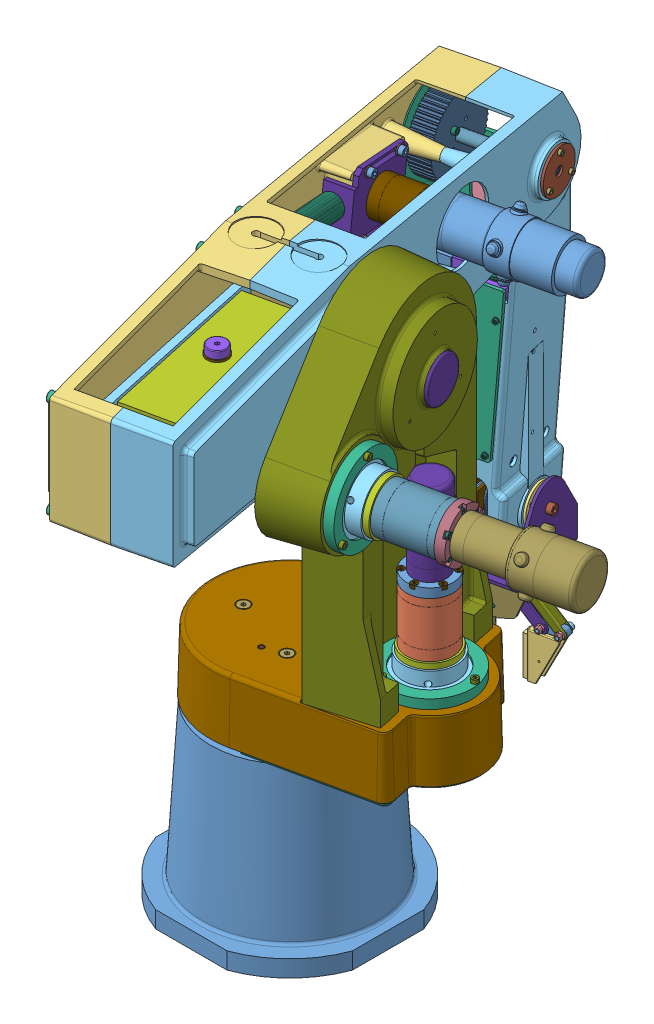
SolidWorks assembly Robot, configuration Défaut. Lengths in mm. (continued)
Components (placement in the parent): (continued)
- SE-AvtBras-1: SE-AvtBras [Défaut] at (-61.3918 532.5 -273.1877) x (0 1 0) z (-0.977211 0 0.212271) size (419.1 115.2 105.3)
  - AvtBrasD-1: AvtBrasD [Défaut] at origin size (406.26 90.38 52)
  - AvtBrasG-1: AvtBrasG [Défaut] at (-0.1665 0.8325 0) size (406.15 90.36 52)
  - parallel pin hardened_iso-1: parallel pin hardened_iso [Goupille  - 4 x 16 - A - St] at (-265.5 30.1675 -8) x (0 0 1) z (-0.010471 -0.999945 0) size (16 4 4)
  - Vis C HC, M 6x70-1: Vis C HC, M 6x70 [Défaut] at (-65 -16 45.5) x (1 0 0) z (0 -1 0) size (10 76 10)
  - GoupillePosition-1: GoupillePosition [Défaut] at (-65 -16 0.2) x (0 0 1) z (-0.991523 0.129934 0) size (10 8 8)
  - Support moteur-1: Support moteur [Défaut] at (-98.931 38.4675 -40.5) x (0 0 1) z (1 0 0) size (77 78 106)
  - socket head cap screw_iso-1: socket head cap screw_iso [Vis CHC M5 x 12 --- 12N] at (-173.5 -4.3325 -27.8) x (0 0 -1) z (0.120643 0.992696 0) size (17 8.5 8.5)
  - socket head cap screw_iso-2: socket head cap screw_iso [Vis CHC M5 x 12 --- 12N] at (-153.5 -4.3325 -27.8) x (0 0 -1) z (0.975756 0.218862 0) size (17 8.5 8.5)
  - plain washer large grade ac_iso-1: plain washer large grade ac_iso [Rondelle M5 Washer ISO 7093 - 5] at (-173.5 -4.3325 -32.8) x (0 0 1) z (-1 0 0) size (1.2 15 15)
  - plain washer large grade ac_iso-3: plain washer large grade ac_iso [Rondelle M5 Washer ISO 7093 - 5] at (-153.5 -4.3325 -32.8) x (0 0 1) z (-1 0 0) size (1.2 15 15)
  - Poulie_M300-006-1: Poulie_M300-006 [Défaut] at (0 0 39) x (0 0 1) z (-0.707107 -0.707107 0) size (22 81.46 81.46)
  - Goupille Cylindrique type A  , 4x24-1: Goupille Cylindrique type A  , 4x24 [Défaut] at (9.1924 9.1924 26.3203) x (0.697271 -0.716808 0) z (0 0 1) size (4 4 24)
  - Goupille Cylindrique type A  , 4x24-3: Goupille Cylindrique type A  , 4x24 [Défaut] at (-9.1924 -9.1924 24.7225) x (-0.993131 -0.117006 0) z (0 0 1) size (4 4 24)
  - socket head cap screw_iso-3: socket head cap screw_iso [Vis CHC M4 x 25 ] at (-9.1924 9.1924 20) x (0 0 1) z (-1 0 0) size (29 7 7)
  - socket head cap screw_iso-4: socket head cap screw_iso [Vis CHC M4 x 25 ] at (9.1924 -9.1924 20) x (0 0 1) z (-1 0 0) size (29 7 7)
  - Came M300 008-1: Came M300 008 [Default] at (0 0 -43) x (0.999885 0.015178 0) z (0 0 1) size (76.42 80 10)
  - parallel pin hardened_iso-2: parallel pin hardened_iso [Goupille  - 4 x 16 - A - St] at (-6.5 -11.2583 -51.3276) x (0 0 1) z (-0.969957 0.243275 0) size (16 4 4)
  - socket head cap screw_iso-5: socket head cap screw_iso [CHC M4 x 16 --- 16N] at (-12.9985 -0.1973 -29) x (0 0 -1) z (-0.999639 0.026878 0) size (20 7 7)
  - socket head cap screw_iso-10: socket head cap screw_iso [CHC M4 x 16 --- 16N] at (6.6701 -11.1584 -29) x (0 0 -1) z (-0.999639 0.026878 0) size (20 7 7)
  - socket head cap screw_iso-12: socket head cap screw_iso [CHC M4 x 16 --- 16N] at (6.3284 11.3557 -29) x (0 0 -1) z (-0.999639 0.026878 0) size (20 7 7)
  - plain washer small grade a_iso-1: plain washer small grade a_iso [Washer M 4] at (-265.5 -21.8325 -8) x (0 0 1) z (-1 0 0) size (0.5 8 8)
  - socket head cap screw_iso-18: socket head cap screw_iso [CHC M4 x 16 --- 16N] at (-265.5 -21.8325 -12.5) x (0 0 1) z (-1 0 0) size (20 7 7)
  - plain washer small grade a_iso-3: plain washer small grade a_iso [Washer M 4] at (-265.5 23.1675 -8) x (0 0 1) z (-1 0 0) size (0.5 8 8)
  - socket head cap screw_iso-19: socket head cap screw_iso [CHC M4 x 16 --- 16N] at (-265.5 23.1675 -12.5) x (0 0 1) z (-1 0 0) size (20 7 7)
  - plain washer small grade a_iso-5: plain washer small grade a_iso [Washer M 4] at (-43.253 27.1675 -8) x (0 0 1) z (-1 0 0) size (0.5 8 8)
  - socket head cap screw_iso-20: socket head cap screw_iso [CHC M4 x 16 --- 16N] at (-43.253 27.1675 -12.5) x (0 0 1) z (-1 0 0) size (20 7 7)
  - moteur poignet-1: moteur poignet [Défaut] at (-218.4709 19.4675 19.5) size (70.8 35 35)
  - socket head cap screw_iso-21: socket head cap screw_iso [ISO 4762 M2 x 6 --- 6N] at (-174.931 8.4675 19.5) x (-1 0 0) z (0 0.924225 0.381849) size (8 3.8 3.8)
  - socket head cap screw_iso-22: socket head cap screw_iso [ISO 4762 M2 x 6 --- 6N] at (-174.931 19.4675 8.5) x (-1 0 0) z (0 -0.381849 0.924225) size (8 3.8 3.8)
  - socket head cap screw_iso-23: socket head cap screw_iso [ISO 4762 M2 x 6 --- 6N] at (-174.931 30.4675 19.5) x (-1 0 0) z (0 -0.924225 -0.381849) size (8 3.8 3.8)
  - socket head cap screw_iso-24: socket head cap screw_iso [ISO 4762 M2 x 6 --- 6N] at (-174.931 19.4675 30.5) x (-1 0 0) z (0 0.381849 -0.924225) size (8 3.8 3.8)
  - Vis CS, M 4x55-1: Vis CS, M 4x55 [Défaut] at (-88.5 -0.5325 -38.5) x (0 -1 0) z (0 0 1) size (7 57.41 7)
  - hex thin nut gradeb_iso-1: hex thin nut gradeb_iso [Hexagon Nut ISO - 4036 - M4 - N] at (-96.731 -0.5325 -38.5) x (0 -0.306361 -0.951915) z (1 0 0) size (7 8.08 2.2)
  - Accouplement flexible-1: Accouplement flexible [Default] at (-161.451 19.4675 19.5) x (-1 0 0) z (0 0.117803 -0.993037) size (17.76 9.53 9.53)
  - Codeur poignet-1: Codeur poignet [Défaut] at (-230.631 -7.9406 32.9669) x (0 0.056728 -0.99839) z (1 0 0) size (30 41.1 18.3)
  - Réducteur-1: Réducteur [Défaut] at (-143.931 29.4675 5.5) x (1 0 0) z (0 0 -1) size (82 70 28)
  - radial ball bearing_68_iso-1: radial ball bearing_68_iso [RBB - 1810 - 14,SI,NC,14_68] at (-317.5 -0.8325 -38.5) x (0 0 1) z (-0.812829 -0.582503 0) size (5 19 19)
  - plain washer small grade a_iso-6: plain washer small grade a_iso [Washer courte m5 7092 - 5] at (-138.931 7.4675 33.5) x (0 0 -1) z (1 0 0) size (1 9 9)
  - socket head cap screw_iso-25: socket head cap screw_iso [vis chc M5 x 35 --- 22N] at (-138.931 7.4675 39.5) x (0 0 -1) z (0.75446 0.656346 0) size (40 8.5 8.5)
  - plain washer small grade a_iso-7: plain washer small grade a_iso [Washer courte m5 7092 - 5] at (-88.931 7.4675 33.5) x (0 0 -1) z (1 0 0) size (1 9 9)
  - plain washer small grade a_iso-8: plain washer small grade a_iso [Washer courte m5 7092 - 5] at (-88.931 -35.5325 33.5) x (0 0 -1) z (1 0 0) size (1 9 9)
  - socket head cap screw_iso-26: socket head cap screw_iso [vis chc M5 x 35 --- 22N] at (-88.931 7.4675 39.5) x (0 0 -1) z (0.75446 0.656346 0) size (40 8.5 8.5)
  - socket head cap screw_iso-27: socket head cap screw_iso [vis chc M5 x 35 --- 22N] at (-88.931 -35.5325 39.5) x (0 0 -1) z (0.75446 0.656346 0) size (40 8.5 8.5)
  - Couvercle-3: Couvercle [Défaut] at (-317.5 -0.8325 -49.8) x (-0.559761 -0.828654 0) z (-0.828654 0.559761 0) size (41 8.8 41)
  - socket head cap screw_iso-28: socket head cap screw_iso [Vis CHC M3x8] at (-310.5 11.2918 -52.8) x (0 0 1) z (-0.923728 -0.383049 0) size (11 5.5 5.5)
  - socket head cap screw_iso-29: socket head cap screw_iso [Vis CHC M3x8] at (-310.5 -12.9569 -52.8) x (0 0 1) z (0.130134 0.991496 0) size (11 5.5 5.5)
  - socket head cap screw_iso-30: socket head cap screw_iso [Vis CHC M3x8] at (-331.5 -0.8325 -52.8) x (0 0 1) z (0.793594 -0.608447 0) size (11 5.5 5.5)
  - radial ball bearing_68_iso-4: radial ball bearing_68_iso [RBB - 1810 - 14,SI,NC,14_68] at (-317.5 -0.8325 38.2) x (0 0 1) z (-0.978908 -0.204302 0) size (5 19 19)
  - Couvercle-4: Couvercle [Défaut] at (-317.5 -0.8325 49.5) x (0.997516 0.070441 0) z (-0.070441 0.997516 0) size (41 8.8 41)
  - socket head cap screw_iso-31: socket head cap screw_iso [Vis CHC M3x8] at (-310.5 11.2918 52.5) x (0 0 -1) z (1 0 0) size (11 5.5 5.5)
  - socket head cap screw_iso-32: socket head cap screw_iso [Vis CHC M3x8] at (-331.5 -0.8325 52.5) x (0 0 -1) z (-0.5 0.866025 0) size (11 5.5 5.5)
  - socket head cap screw_iso-33: socket head cap screw_iso [Vis CHC M3x8] at (-310.5 -12.9569 52.5) x (0 0 -1) z (-0.5 -0.866025 0) size (11 5.5 5.5)
  - Capot Superieur_plexi-1: Capot Superieur_plexi [Défaut] at (-81.8928 43.8087 0) x (1 0 0) z (0 1 0) size (220 89.9 3.57)
  - plain washer 10673 type snl_iso-1: plain washer 10673 type snl_iso [rondelle M2] at (-264 46.4087 28) x (0 -1 0) z (0 0 1) size (0.6 6 6)
  - socket head cap screw_iso-34: socket head cap screw_iso [ISO 4762 M2.5 x 10 --- 10N] at (-264 48.9087 28) x (0 -1 0) z (0 0 1) size (12.5 4.5 4.5)
  - plain washer 10673 type snl_iso-9: plain washer 10673 type snl_iso [rondelle M2] at (-264 46.4087 -28) x (0 -1 0) z (0 0 1) size (0.6 6 6)
  - plain washer 10673 type snl_iso-11: plain washer 10673 type snl_iso [rondelle M2] at (-54 46.4087 -40) x (0 -1 0) z (0 0 1) size (0.6 6 6)
  - plain washer 10673 type snl_iso-13: plain washer 10673 type snl_iso [rondelle M2] at (-54 46.4087 40) x (0 -1 0) z (0 0 1) size (0.6 6 6)
  - socket head cap screw_iso-35: socket head cap screw_iso [ISO 4762 M2.5 x 10 --- 10N] at (-264 48.9087 -28) x (0 -1 0) z (0 0 1) size (12.5 4.5 4.5)
  - socket head cap screw_iso-36: socket head cap screw_iso [ISO 4762 M2.5 x 10 --- 10N] at (-54 48.9087 -40) x (0 -1 0) z (0 0 1) size (12.5 4.5 4.5)
  - socket head cap screw_iso-37: socket head cap screw_iso [ISO 4762 M2.5 x 10 --- 10N] at (-54 48.9087 40) x (0 -1 0) z (0 0 1) size (12.5 4.5 4.5)
  - Capot inferieur_plexi-1: Capot inferieur_plexi [Défaut] at (-207.8847 -47.4738 0) x (1 0 0) z (0 1 0) size (165 92.79 3.62)
  - plain washer 10673 type snl_iso-14: plain washer 10673 type snl_iso [rondelle M2] at (-121.3236 -48.0738 -40) x (0 1 0) z (-1 0 0) size (0.6 6 6)
  - plain washer 10673 type snl_iso-16: plain washer 10673 type snl_iso [rondelle M2] at (-121.3236 -48.0738 40) x (0 1 0) z (-1 0 0) size (0.6 6 6)
  - plain washer 10673 type snl_iso-18: plain washer 10673 type snl_iso [rondelle M2] at (-251.3236 -48.0738 30) x (0 1 0) z (-1 0 0) size (0.6 6 6)
  - plain washer 10673 type snl_iso-20: plain washer 10673 type snl_iso [rondelle M2] at (-251.3236 -48.0738 -30) x (0 1 0) z (-1 0 0) size (0.6 6 6)
  - socket head cap screw_iso-38: socket head cap screw_iso [ISO 4762 M2.5 x 10 --- 10N] at (-251.3236 -50.5738 -30) x (0 1 0) z (0 0 1) size (12.5 4.5 4.5)
  - socket head cap screw_iso-39: socket head cap screw_iso [ISO 4762 M2.5 x 10 --- 10N] at (-251.3236 -50.5738 30) x (0 1 0) z (0 0 -1) size (12.5 4.5 4.5)
  - socket head cap screw_iso-40: socket head cap screw_iso [ISO 4762 M2.5 x 10 --- 10N] at (-121.3236 -50.5738 40) x (0 1 0) z (0 0 -1) size (12.5 4.5 4.5)
  - socket head cap screw_iso-41: socket head cap screw_iso [ISO 4762 M2.5 x 10 --- 10N] at (-121.3236 -50.5738 -40) x (0 1 0) z (0 0 -1) size (12.5 4.5 4.5)
  - radial ball bearing_68_skf-1: radial ball bearing_68_skf [Roulement à billes 618-8] at (-113.931 -10.5325 -32.5) x (0 0 -1) z (1 0 0) size (4 16 16)
  - Arbre réducteur-1: Arbre réducteur [Défaut] at (-113.931 -10.5325 33.5) size (8 8 68)
  - Entretoise-1: Entretoise [Défaut] at (-113.931 -10.5325 -10.5) size (12 12 16)
- Arbre moteur Lacet-1: Arbre moteur Lacet [Défaut] at (122.0871 255.5 -29.1721) x (0 -1 0) z (-0.495579 0 0.868563) size (78.5 36.84 36.92)
  - entraineur-1: entraineur [Défaut] at origin size (78.5 20 20)
  - PoulieE lacet-1: PoulieE lacet [Défaut] at (49 0 0) x (0 -1 0) z (-1 0 0) size (36.84 36.92 30)
  - socket set screw flat point_iso-1: socket set screw flat point_iso [ISO 4026 - M8 x 10-N] at (49 0 16.5) x (0 0 -1) z (1 0 0) size (10 8 8)
  - socket set screw flat point_iso-2: socket set screw flat point_iso [ISO 4026 - M8 x 10-N] at (-7.2554 0 12.9535) x (0 0 -1) z (0.96252 -0.271209 0) size (10 8 8)
- A-M_Epaule-1: A-M_Epaule [Défaut] at (143.3488 474.5 66.3524) x (-0.977211 0 0.212271) z (-0.212271 0 -0.977211) size (78.5 36.84 36.92)
  - entraineur-1: entraineur [Défaut] at origin size (78.5 20 20)
  - P-E_Epaule-1: P-E_Epaule [Défaut] at (49 0 0) x (0 -1 0) z (-1 0 0) size (36.84 36.92 30)
  - socket set screw flat point_iso-1: socket set screw flat point_iso [ISO 4026 - M8 x 10-N] at (49 0 16.5) x (0 0 -1) z (1 0 0) size (10 8 8)
  - socket set screw flat point_iso-2: socket set screw flat point_iso [ISO 4026 - M8 x 10-N] at (-7.2554 0 12.9535) x (0 0 -1) z (0.96252 -0.271209 0) size (10 8 8)
- Poulie_M300-007-1: Poulie_M300-007 [Défaut] at (-55.3873 549.2909 -151.3264) x (0.977211 0 -0.212271) z (0.17106 -0.592111 0.787492) size (27 22.5 22.65)
- Poulie Poignet-1: Poulie Poignet [Défaut] at (-39.1232 418.569 -267.2467) x (-0.212271 0 -0.977211) z (0.977211 0 -0.212271) size (27.43 27.43 20)
- poulie pivotement poignet-1: poulie pivotement poignet [Défaut] at (-76.1895 174.3879 -240.3141) x (-0.99945 0 0.033175) z (0 -1 0) size (20 20 14)
- Support_poignet-1: Support_poignet [Défaut] at (-61.215 215 -272.3741) x (0 1 0) z (-0.977211 0 0.212271) size (98.66 84.05 127)
  - Support-1: Support [Défaut] at origin size (81.5 81.2 115)
  - Assemblage axe pince-1: Assemblage axe pince [Défaut] at (-13.5 0 0) x (0 0 -1) z (1 0 0) size (109 40 59)
    - partie centrale axe avant bras-1: partie centrale axe avant bras [Défaut] at origin size (12 40 21)
    - intérieur pièce centrale-1: intérieur pièce centrale [Défaut] at (-3 1.5 5) size (6 15.94 13)
    - intérieur pièce centrale-2: intérieur pièce centrale [Défaut] at (3 -1.5 5) x (-1 0 0) z (0 0 1) size (6 15.94 13)
    - coté axe avant bras-1: coté axe avant bras [Défaut] at (-6 1.807 8.3053) x (1 0 0) z (0 0.944488 0.328546) size (48.5 11 11)
    - coté axe avant bras-2: coté axe avant bras [Défaut] at (6 -1.6292 8.2468) x (-1 0 0) z (0 -0.95512 0.296219) size (48.5 11 11)
    - axe roulements-1: axe roulements [Défaut] x (0 0 -1) z (0.989499 0.144542 0) size (38 10.89 10.89)
  - Assemblage support moteur-1: Assemblage support moteur [Défaut] at (-44.3507 -38.7833 30.5386) x (-1 0 0) z (0 0 -1) size (78.32 60.15 22.52)
    - Support moteur + axe-1: Support moteur + axe [Défaut] at origin size (75.82 60.15 22.2)
    - capteur sur support moteur-1: capteur sur support moteur [Défaut] at (-40.0112 47.5459 15.95) x (0 -0.781659 -0.623706) z (1 0 0) size (6.5 6.5 27.6)
    - plaque avant support moteur-1: plaque avant support moteur [Défaut] at (14.8869 1.1807 -1.9) x (0 0 -1) z (1 0 0) size (22 24 2.5)
  - Ecrou hexagonal ISO 4032, M 9-1: Ecrou hexagonal ISO 4032, M 9 [Défaut] at (-44.23 0 0) x (0 1 0) z (0 0 1) size (16.17 6.98 14)
  - moteur pivotement poignet-1: moteur pivotement poignet [Défaut] at (-26.4843 -28.1507 21.4386) x (-1 0 0) z (0 -0.157023 -0.987595) size (81.2 19.59 19.59)
    - réducteur micromoteur-1: réducteur micromoteur [Défaut] at origin size (48.3 16 16)
    - micromoteur-1: micromoteur [Défaut] at (-2.1408 0 0) x (1 0 0) z (0 -0.965969 0.258658) size (41 16 16)
  - Poulie axe poignet-1: Poulie axe poignet [Défaut] at (0 0 -18.0612) x (-0.954858 -0.297063 0) z (0 0 -1) size (58.99 58.99 20)
  - Vis C HC, M 6x16-1: Vis C HC, M 6x16 [Défaut] at (0 0 57.5) x (0.243653 -0.969862 0) z (-0.969862 -0.243653 0) size (10 22.04 10)
  - Vis C HC, M 6x16-2: Vis C HC, M 6x16 [Défaut] at (0 0 -57.5) x (1 0 0) z (0 1 0) size (10 22.04 10)
- PortePince-1: PortePince [Défaut] at (-61.215 215 -272.3741) x (0 1 0) z (0.212271 0 0.977211) size (147.79 157.25 45.47)
  - Corps_poignet-1: Corps_poignet [Défaut] at (-113.4 0 -8.5) x (0 -1 0) z (0 0 1) size (87.98 118.07 45.47)
    - Main-1: Main [Défaut] at origin size (87.98 81.17 33)
    - fourreau de poignet-1: fourreau de poignet [Défaut] at (0 76.4 8.5) x (0 1 0) z (0.435216 0 0.900326) size (46.9 34.05 34.05)
    - Roulement type BC 9x17x4-1: Roulement type BC 9x17x4 [Défaut] at (0 94.9 8.5) x (0 -1 0) z (-0.453716 0 0.891146) size (4 17 17)
    - Roulement type BC 9x17x4-2: Roulement type BC 9x17x4 [Défaut] at (0 71.1711 8.5) x (0 -1 0) z (0 0 1) size (4 17 17)
    - Axe-goupille-1: Axe-goupille [Défaut] at (36.5 37 17) size (3.5 3.5 17)
    - Axe-goupille-2: Axe-goupille [Défaut] at (18.5 37 17) size (3.5 3.5 17)
    - Axe-goupille-3: Axe-goupille [Défaut] at (-18.5 37 17) size (3.5 3.5 17)
    - Axe-goupille-4: Axe-goupille [Défaut] at (-36.5 37 17) size (3.5 3.5 17)
    - Axe-goupille-5: Axe-goupille [Défaut] at (-12.5 10 17) size (3.5 3.5 17)
    - Axe-goupille-6: Axe-goupille [Défaut] at (12.5 10 17) size (3.5 3.5 17)
  - bielle 1-1: bielle 1 [Défaut] at (-106.9547 -75.1317 5.4) x (-0.717304 0.69676 0) z (0 0 -1) size (9.87 58.75 10.8)
  - bielle 1-2: bielle 1 [Défaut] at (-106.9547 75.1317 -5.4) x (-0.717304 -0.69676 0) z (0 0 1) size (9.87 58.75 10.8)
  - bielle 2-1: bielle 2 [Défaut] at (-80.8832 -14.1453 5.4) x (0.717304 -0.69676 0) z (0 0 -1) size (12.5 61.5 10.8)
    - bielle 2-1: bielle 2 [Défaut] at origin size (12.5 61.5 10.8)
    - goupille bielle 2-1: goupille bielle 2 [Défaut] at (6.25 18 10.8) x (-0.698934 -0.715186 0) z (0 0 1) size (3.5 3.5 10.8)
  - bielle 2-2: bielle 2 [Défaut] at (-80.8832 14.1453 -5.4) x (0.717304 0.69676 0) z (0 0 1) size (12.5 61.5 10.8)
    - bielle 2-1: bielle 2 [Défaut] at origin size (12.5 61.5 10.8)
    - goupille bielle 2-1: goupille bielle 2 [Défaut] at (6.25 18 10.8) x (-0.698934 -0.715186 0) z (0 0 1) size (3.5 3.5 10.8)
  - Mors-3: Mors [Défaut] at (-210.2541 103.6501 -0.5) x (-1 0 0) z (0 0 -1) size (60 39.8 20)
    - Bielle 3-1: Bielle 3 [Défaut] at (-104.4629 -50.0022 -4.6) size (9.5 27.5 8.2)
    - goupille-1: goupille [Défaut] at (-106.9629 -37.5022 -0.5) x (0 -0.527582 0.849504) z (-1 0 0) size (4 4 14)
    - mors-1: mors [Défaut] at (-49.5801 -64.5882 6.5) size (48 34 14)
    - ecrou_uni_7474-m4x0_7-4_8-5s-1: ecrou_uni_7474-m4x0_7-4_8-5s [Défaut] at (-99.7129 -32.0022 4.9) x (0.66757 0.744547 0) z (0 0 1) size (7 8.09 4.8)
    - ecrou_uni_7474-m4x0_7-4_8-5s-2: ecrou_uni_7474-m4x0_7-4_8-5s [Défaut] at (-99.7129 -50.0022 4.9) x (0.967807 0.251692 0) z (0 0 1) size (7 8.09 4.8)
    - vis chc M4x16-1: vis chc M4x16 [Default] at (-99.7129 -32.0022 -5.9) x (0.255972 0.966684 0) z (0 0 1) size (7 7 20)
    - vis chc M4x16-2: vis chc M4x16 [Default] at (-99.7129 -50.0022 -5.9) x (-0.658187 0.752854 0) z (0 0 1) size (7 7 20)
    - Vis Chc M4-1: Vis Chc M4 [Default] at (-92.9629 -44.5022 -0.5) x (0 0 1) z (-1 0 0) size (7 7 16)
  - Mors-4: Mors [Défaut] at (-210.2541 -103.6501 0.5) x (-1 0 0) z (0 0 1) size (60 39.8 20)
    - Bielle 3-1: Bielle 3 [Défaut] at (-104.4629 -50.0022 -4.6) size (9.5 27.5 8.2)
    - goupille-1: goupille [Défaut] at (-106.9629 -37.5022 -0.5) x (0 -0.527582 0.849504) z (-1 0 0) size (4 4 14)
    - mors-1: mors [Défaut] at (-49.5801 -64.5882 6.5) size (48 34 14)
    - ecrou_uni_7474-m4x0_7-4_8-5s-1: ecrou_uni_7474-m4x0_7-4_8-5s [Défaut] at (-99.7129 -32.0022 4.9) x (0.66757 0.744547 0) z (0 0 1) size (7 8.09 4.8)
    - ecrou_uni_7474-m4x0_7-4_8-5s-2: ecrou_uni_7474-m4x0_7-4_8-5s [Défaut] at (-99.7129 -50.0022 4.9) x (0.967807 0.251692 0) z (0 0 1) size (7 8.09 4.8)
    - vis chc M4x16-1: vis chc M4x16 [Default] at (-99.7129 -32.0022 -5.9) x (0.255972 0.966684 0) z (0 0 1) size (7 7 20)
    - vis chc M4x16-2: vis chc M4x16 [Default] at (-99.7129 -50.0022 -5.9) x (-0.658187 0.752854 0) z (0 0 1) size (7 7 20)
    - Vis Chc M4-1: Vis Chc M4 [Default] at (-92.9629 -44.5022 -0.5) x (0 0 1) z (-1 0 0) size (7 7 16)
Mates (geometry in assembly coordinates):
- Coaxiale1: concentric aligned: cylinder of Ens_Socle-1/Fourreau_200-604-1 through (0 221.7474 0) axis (0 1 0) radius 23.5; cylinder of SE_Chaise-1/SE-Assise-1/SKF_7204-2 through (0 165.3625 0) axis (0 1 0) radius 23.5
- Coïncidente1: coincident anti-aligned: plane of Ens_Socle-1/Fourreau_200-604-1 through (-1.9708 229.5 23.4172) normal (0 -1 0); plane of SE_Chaise-1/SE-Assise-1/SKF_7204-1 through (20.3016 229.5 -4.4099) normal (0 1 0)
- Coaxiale2: concentric anti-aligned: cylinder of SE_Chaise-1/Dossier-1 through (63.5173 532.5 -13.7908) axis (0.977211 0 -0.212271) radius 23.5; cylinder of Bras-1/AXE_Bras-1/7204_Rlt-Billes-2 through (137.9197 532.5 -29.9526) axis (-0.977211 0 0.212271) radius 23.5
- Coïncidente2: coincident anti-aligned: plane of SE_Chaise-1/Dossier-1 through (124.593 532.5 -27.0578) normal (-0.977211 0 0.212271); plane of Bras-1/AXE_Bras-1/7204_Rlt-Billes-2 through (127.5156 548.0575 -13.6033) normal (0.977211 0 -0.212271)
- Coaxiale3: concentric aligned: cylinder of Bras-1/AXE 04 021 M300 011-1 through (-121.9788 532.5 -260.0268) axis (0.977211 0 -0.212271) radius 6; cylinder of SE-AvtBras-1/AvtBrasG-1 through (-112.2067 532.5 -262.1496) axis (0.977211 0 -0.212271) radius 6
- Coïncidente3: coincident aligned: plane of Bras-1/BrasDroit-2 through (-0.5391 505.7717 6.953) normal (-0.977211 0 0.212271); plane of SE-AvtBras-1/AvtBrasD-1 through (-61.3918 532.5 -273.1877) normal (-0.977211 0 0.212271)
- Coaxiale5: concentric aligned: cylinder of SE_Chaise-1/Moto-réducteur lacet-1/SKF 6002-1 through (122.0871 209.2625 -29.1721) axis (0 1 0) radius 7.5; cylinder of Arbre moteur Lacet-1/entraineur-1 through (122.0871 277.7027 -29.1721) axis (0 1 0) radius 7.5
- Coïncidente5: coincident anti-aligned: plane of SE_Chaise-1/Moto-réducteur lacet-1/SKF 6002-2 through (127.3321 255.5 -23.3989) normal (0 1 0); plane of Arbre moteur Lacet-1/entraineur-1 through (130.7727 255.5 -24.2163) normal (0 -1 0)
- Coaxiale6: concentric aligned: cylinder of SE_Chaise-1/Moteur Epaule-1/SKF 6002-2 through (98.165 474.5 76.1673) axis (0.977211 0 -0.212271) radius 7.5; cylinder of A-M_Epaule-1/entraineur-1 through (165.0455 474.5 61.6395) axis (0.977211 0 -0.212271) radius 7.5
- Coïncidente6: coincident anti-aligned: plane of SE_Chaise-1/Moteur Epaule-1/SKF 6002-1 through (144.9823 473.2287 73.8728) normal (0.977211 0 -0.212271); plane of A-M_Epaule-1/entraineur-1 through (143.3488 484.5 66.3524) normal (-0.977211 0 0.212271)
- Coaxiale7: concentric anti-aligned: cylinder of Bras-1/MotoReduc_Coude-1/Sortie reduc-1 through (-54.8986 549.2909 -151.4325) axis (0.977211 0 -0.212271) radius 5; cylinder of Poulie_M300-007-1 through (-67.3627 549.2909 -148.725) axis (-0.977211 0 0.212271) radius 5
- Coaxiale8: concentric aligned: cylinder of Bras-1/MotoReduc_Coude-1/Sortie reduc-1 through (-71.8779 552.2514 -151.8675) axis (0.17106 -0.592111 0.787492) radius 1.5; cylinder of Poulie_M300-007-1 through (-72.9599 555.9965 -156.8484) axis (0.17106 -0.592111 0.787492) radius 1.5
- Coaxiale9: concentric aligned: cylinder of SE-AvtBras-1/Arbre réducteur-1 through (-25.4422 418.569 -270.2185) axis (-0.977211 0 0.212271) radius 4; cylinder of Poulie Poignet-1 through (-29.3511 418.569 -269.3694) axis (-0.977211 0 0.212271) radius 4
- Coïncidente7: coincident anti-aligned: plane of SE-AvtBras-1/Entretoise-1 through (-48.8953 418.569 -265.124) normal (0.977211 0 -0.212271); plane of Poulie Poignet-1 through (-48.8953 418.569 -265.124) normal (-0.977211 0 0.212271)
- Coaxiale10: concentric anti-aligned: cylinder of Support_poignet-1/Assemblage axe pince-1/axe roulements-1 through (-61.215 163.5 -272.3741) axis (0 1 0) radius 4.5; cylinder of PortePince-1/Corps_poignet-1/fourreau de poignet-1 through (-61.215 146.4624 -272.3741) axis (0 -1 0) radius 11
- Coaxiale11: concentric anti-aligned: cylinder of Support_poignet-1/Assemblage axe pince-1/coté axe avant bras-2 through (-26.0354 215 -280.0159) axis (0.977211 0 -0.212271) radius 5; cylinder of SE-AvtBras-1/radial ball bearing_68_iso-1 through (-3.4252 215 -284.9273) axis (-0.977211 0 0.212271) radius 5
- Coïncidente8: coincident aligned: plane of SE-AvtBras-1/AvtBrasD-1 through (-61.3918 532.5 -273.1877) normal (-0.977211 0 0.212271); plane of Support_poignet-1/Support-1 through (-61.215 215 -272.3741) normal (-0.977211 0 0.212271)
- Coïncidente9: coincident anti-aligned: plane of Support_poignet-1/Assemblage axe pince-1/axe roulements-1 through (-61.215 198.5 -272.3741) normal (0 -1 0); plane of PortePince-1/Corps_poignet-1/Roulement type BC 9x17x4-1 through (-56.476 198.5 -271.1285) normal (0 1 0)
- Coaxiale12: concentric aligned: cylinder of poulie pivotement poignet-1 through (-76.1895 162.3879 -240.3141) axis (0 1 0) radius 1.5; cylinder of Support_poignet-1/moteur pivotement poignet-1/réducteur micromoteur-1 through (-76.1895 253.1757 -240.3141) axis (0 1 0) radius 1.5
- Coïncidente10: coincident anti-aligned: plane of poulie pivotement poignet-1 through (-76.1895 174.3879 -240.3141) normal (0 1 0); plane of Support_poignet-1/moteur pivotement poignet-1/réducteur micromoteur-1 through (-76.3644 174.3879 -243.4208) normal (0 -1 0)
- Parallèle3: parallel anti-aligned: plane of Ens_Socle-1/Socle-1 through (-113 0 0) normal (0 -1 0); plane of Bras-1/BrasDroit-2
- Parallèle2: parallel aligned: plane of SE-AvtBras-1/AvtBrasD-1; plane of Support_poignet-1/Support-1
- Perpendiculaire1: perpendicular: plane of Ens_Socle-1/Socle-1 through (-113 0 0) normal (0 -1 0); plane of SE-AvtBras-1/AvtBrasD-1
- Coïncidente16: coincident anti-aligned: plane of Support_poignet-1/Support-1; plane of PortePince-1 through (-61.215 215 -272.3741) normal (0.212271 0 0.977211)
